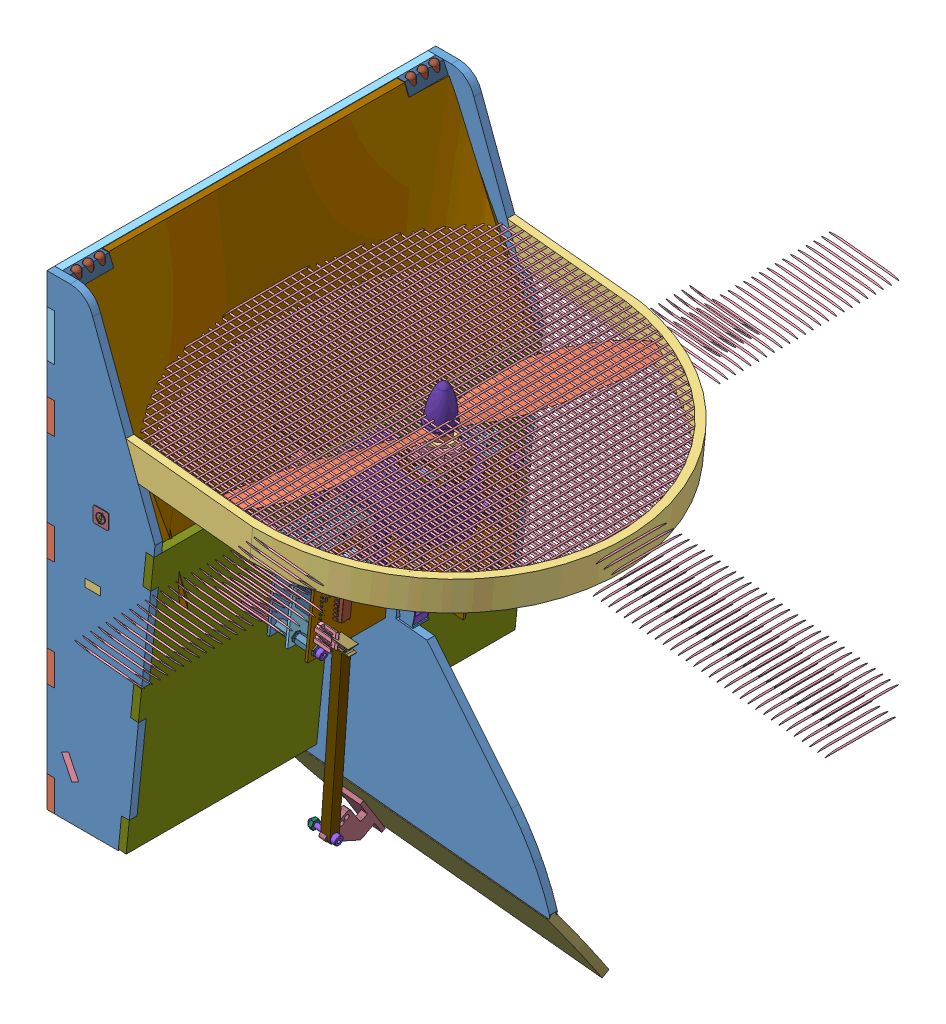
SolidWorks assembly AssTotaleSimu5, configuration Défaut. Lengths in mm. (continued)
Components (placement in the parent): (continued)
- AssStructSimu-1: AssStructSimu [Défaut] at (-125.7658 -1.8483 624.6548) x (1 0 0) z (0 0 -1) size (253.25 324.59 251.6) (continued)
  - AssCarte-1: AssCarte [Défaut] at (38.0121 147.1029 290.772) x (-0.101852 0.9948 0) z (0.9948 0.101852 0) size (66.52 130.57 98.72) (continued)
    - carte_onduleur_v3-1: carte_onduleur_v3 [Défaut] at (-131.8199 12.0892 20.7912) size (66.52 130.57 82.34) (continued)
      - RC2_2-1: RC2_2 [Défaut] at (-22 0.18 -0.803) x (-1 0 0) z (0 0 -1) size (2.34 1.04 0.5) (continued)
        - Open CASCADE STEP translator 6.8 1.12.1-1: Open CASCADE STEP translator 6.8 1.12.1 [Défaut] at origin size (2.34 1.04 0.5) (continued)
          - Pin_2_2-1: Pin_2_2 [Défaut] at origin size (0.51 1.02 0.5)
      - RC3_1-1: RC3_1 [Défaut] at (-20.9336 -14.5 -0.803) x (1 0 0) z (0 0 -1) size (2.34 1.04 0.5)
        - Open CASCADE STEP translator 6.8 1.12.1-1: Open CASCADE STEP translator 6.8 1.12.1 [Défaut] at origin size (2.34 1.04 0.5)
          - Body_1_3-1: Body_1_3 [Défaut] at origin size (2.29 1.04 0.43)
          - Pin_1_2-1: Pin_1_2 [Défaut] at (0.3048 0 0) x (-1 0 0) z (0 0 1) size (0.51 1.02 0.5)
          - Pin_2_2-1: Pin_2_2 [Défaut] at origin size (0.51 1.02 0.5)
      - RC3_2-1: RC3_2 [Défaut] at (-22.3 -14.5 -0.803) x (-1 0 0) z (0 0 -1) size (2.34 1.04 0.5)
        - Open CASCADE STEP translator 6.8 1.12.1-1: Open CASCADE STEP translator 6.8 1.12.1 [Défaut] at origin size (2.34 1.04 0.5)
          - Body_1_3-1: Body_1_3 [Défaut] at origin size (2.29 1.04 0.43)
          - Pin_1_2-1: Pin_1_2 [Défaut] at (0.3048 0 0) x (-1 0 0) z (0 0 1) size (0.51 1.02 0.5)
          - Pin_2_2-1: Pin_2_2 [Défaut] at origin size (0.51 1.02 0.5)
      - U_MES_CUR-1: U_MES_CUR [Défaut] at (-11.5 6.7816 0.803) size (2.54 2.41 0.76)
        - Open CASCADE STEP translator 6.8 1.32.1-1: Open CASCADE STEP translator 6.8 1.32.1 [Défaut] at origin size (2.54 2.41 0.76)
          - Body_1_5-1: Body_1_5 [Défaut] at origin size (2.54 1.27 0.71)
          - Pin_1_3-1: Pin_1_3 [Défaut] at (-2.1082 0.2286 0) x (0 -1 0) z (0 0 1) size (1.14 0.25 0.47)
          - Pin_2_3-1: Pin_2_3 [Défaut] at (-0.2032 2.1336 0) x (0 -1 0) z (0 0 1) size (1.14 0.25 0.47)
      - CARTE_ALIM-1: CARTE_ALIM [Défaut] at (-6.4 -57.2 0.803) size (60 130 18.35)
        - Open CASCADE STEP translator 6.8 1.33.1-1: Open CASCADE STEP translator 6.8 1.33.1 [Défaut] at origin size (60 130 18.35)
          - Body_1_6-1: Body_1_6 [Défaut] at (7 56 -12) size (60 130 18.35)
            - 1_3-1: 1_3 [Défaut] at origin size (60 130 1.61)
            - 13_3-1: 13_3 [Défaut] at (0.4717 -40.93 0.803) x (0 1 0) z (0 0 1) size (5.65 4.9 1.7)
              - =_[0_1_1_4]_3-1: =_[0_1_1_4]_3 [Défaut] at origin size (5.65 4.9 1.7)
                - 2-1: 2 [Défaut] at origin size (3.75 4.9 1.53)
                - 3-1: 3 [Défaut] at origin size (0.95 0.51 1.06)
                - 4-1: 4 [Défaut] at origin size (0.95 0.51 1.06)
                - 5_2-1: 5_2 [Défaut] at origin size (0.95 0.51 1.06)
                - 6-1: 6 [Défaut] at origin size (0.95 0.51 1.06)
                - 7-1: 7 [Défaut] at (10.8 -5.08 0) x (-1 0 0) z (0 0 1) size (0.95 0.51 1.06)
                - 8_2-1: 8_2 [Défaut] at (10.8 -2.54 0) x (-1 0 0) z (0 0 1) size (0.95 0.51 1.06)
                - 9-1: 9 [Défaut] at (10.8 0 0) x (-1 0 0) z (0 0 1) size (0.95 0.51 1.06)
                - 10-1: 10 [Défaut] at (10.8 2.54 0) x (-1 0 0) z (0 0 1) size (0.95 0.51 1.06)
                - 11_2-1: 11_2 [Défaut] at (5.4 -1.27 0) x (-1 0 0) z (0 0 1) size (4.25 2.34 1.06)
            - 18-1: 18 [Défaut] at (-2.5283 -37.23 0.803) x (0 -1 0) z (0 0 1) size (2.34 1.04 0.5)
              - =_[0_1_1_16]-1: =_[0_1_1_16] [Défaut] at origin size (2.34 1.04 0.5)
                - 14_2-1: 14_2 [Défaut] at origin size (2.29 1.04 0.43)
                - 15_2-1: 15_2 [Défaut] at (0.3048 0 0) x (-1 0 0) z (0 0 1) size (0.51 1.02 0.5)
                - 16_2-1: 16_2 [Défaut] at origin size (0.51 1.02 0.5)
            - 21_2-1: 21_2 [Défaut] at (-2.2263 -24.628 -0.803) x (1 0 0) z (0 0 -1) size (8.01 8 14.24)
              - =_[0_1_1_21]-1: =_[0_1_1_21] [Défaut] at origin size (8.01 8 14.24)
                - 19-1: 19 [Défaut] at (1.8 0 0) x (1 0 0) z (0 -1 0) size (8.01 14.24 8)
            - 23_2-1: 23_2 [Défaut] at (1.2381 -31.53 0.803) size (2.34 1.04 0.5)
              - =_[0_1_1_16]-1: =_[0_1_1_16] [Défaut] at origin size (2.34 1.04 0.5)
                - 14_2-1: 14_2 [Défaut] at origin size (2.29 1.04 0.43)
                - 15_2-1: 15_2 [Défaut] at (0.3048 0 0) x (-1 0 0) z (0 0 1) size (0.51 1.02 0.5)
                - 16_2-1: 16_2 [Défaut] at origin size (0.51 1.02 0.5)
            - 28-1: 28 [Défaut] at (5 29.8636 0.803) x (0 -1 0) z (0 0 1) size (3.35 1.3 0.55)
              - =_[0_1_1_25]_2-1: =_[0_1_1_25]_2 [Défaut] at origin size (3.35 1.3 0.55)
                - 24-1: 24 [Défaut] at origin size (3.3 1.3 0.48)
                - 25_2-1: 25_2 [Défaut] at (0.5588 0 0) x (-1 0 0) z (0 0 1) size (0.76 1.27 0.55)
                - 26_2-1: 26_2 [Défaut] at origin size (0.76 1.27 0.55)
            - 30-1: 30 [Défaut] at (6.7 29.8636 0.803) x (0 -1 0) z (0 0 1) size (2.34 1.04 0.5)
              - =_[0_1_1_16]-1: =_[0_1_1_16] [Défaut] at origin size (2.34 1.04 0.5)
                - 14_2-1: 14_2 [Défaut] at origin size (2.29 1.04 0.43)
                - 15_2-1: 15_2 [Défaut] at (0.3048 0 0) x (-1 0 0) z (0 0 1) size (0.51 1.02 0.5)
                - 16_2-1: 16_2 [Défaut] at origin size (0.51 1.02 0.5)
            - 35_2-1: 35_2 [Défaut] at (-2.5 -46.37 0.803) x (0 1 0) z (0 0 1) size (3.4 2.06 0.79)
              - =_[0_1_1_31]-1: =_[0_1_1_31] [Défaut] at origin size (3.4 2.06 0.79)
                - 31_2-1: 31_2 [Défaut] at origin size (3.3 2.06 0.69)
                - 32_3-1: 32_3 [Défaut] at (0.5588 0 0) x (-1 0 0) z (0 0 1) size (0.81 2.03 0.79)
                - 33_3-1: 33_3 [Défaut] at origin size (0.81 2.03 0.79)
            - 37-1: 37 [Défaut] at (5 31.43 0.803) x (0 1 0) z (0 0 1) size (2.34 1.04 0.5)
              - =_[0_1_1_16]-1: =_[0_1_1_16] [Défaut] at origin size (2.34 1.04 0.5)
                - 14_2-1: 14_2 [Défaut] at origin size (2.29 1.04 0.43)
                - 15_2-1: 15_2 [Défaut] at (0.3048 0 0) x (-1 0 0) z (0 0 1) size (0.51 1.02 0.5)
                - 16_2-1: 16_2 [Défaut] at origin size (0.51 1.02 0.5)
            - 39-1: 39 [Défaut] at (-0.2 35.63 0.803) x (-1 0 0) z (0 0 1) size (2.34 1.04 0.5)
              - =_[0_1_1_16]-1: =_[0_1_1_16] [Défaut] at origin size (2.34 1.04 0.5)
                - 14_2-1: 14_2 [Défaut] at origin size (2.29 1.04 0.43)
                - 15_2-1: 15_2 [Défaut] at (0.3048 0 0) x (-1 0 0) z (0 0 1) size (0.51 1.02 0.5)
                - 16_2-1: 16_2 [Défaut] at origin size (0.51 1.02 0.5)
            - 41-1: 41 [Défaut] at (2.9 -45.5036 0.803) x (0 1 0) z (0 0 1) size (2.34 1.04 0.5)
              - =_[0_1_1_16]-1: =_[0_1_1_16] [Défaut] at origin size (2.34 1.04 0.5)
                - 14_2-1: 14_2 [Défaut] at origin size (2.29 1.04 0.43)
                - 15_2-1: 15_2 [Défaut] at (0.3048 0 0) x (-1 0 0) z (0 0 1) size (0.51 1.02 0.5)
                - 16_2-1: 16_2 [Défaut] at origin size (0.51 1.02 0.5)
            - 43-1: 43 [Défaut] at (17.1348 -42.6272 0.803) x (0 1 0) z (0 0 1) size (2.34 1.04 0.5)
              - =_[0_1_1_16]-1: =_[0_1_1_16] [Défaut] at origin size (2.34 1.04 0.5)
                - 14_2-1: 14_2 [Défaut] at origin size (2.29 1.04 0.43)
                - 15_2-1: 15_2 [Défaut] at (0.3048 0 0) x (-1 0 0) z (0 0 1) size (0.51 1.02 0.5)
                - 16_2-1: 16_2 [Défaut] at origin size (0.51 1.02 0.5)
            - 48_2-1: 48_2 [Défaut] at (-5.4717 -39.01 0.803) x (-1 0 0) z (0 0 1) size (4.19 3.4 1.75)
              - =_[0_1_1_40]-1: =_[0_1_1_40] [Défaut] at origin size (4.19 3.4 1.75)
                - 44_2-1: 44_2 [Défaut] at origin size (3.75 3.38 1.73)
                - 45_2-1: 45_2 [Défaut] at (0.438 0 0) x (-1 0 0) z (0 0 1) size (0.53 3.4 1.75)
                - 46_2-1: 46_2 [Défaut] at origin size (0.52 3.4 1.75)
            - 53-1: 53 [Défaut] at (0.9 35.63 0.803) size (2.34 1.04 0.5)
              - =_[0_1_1_45]-1: =_[0_1_1_45] [Défaut] at origin size (2.34 1.04 0.5)
                - 49_3-1: 49_3 [Défaut] at origin size (2.29 1.04 0.43)
                - 50-1: 50 [Défaut] at (0.3048 0 0) x (-1 0 0) z (0 0 1) size (0.51 1.02 0.5)
                - 51-1: 51 [Défaut] at origin size (0.51 1.02 0.5)
            - 55_2-1: 55_2 [Défaut] at (1.3 -45.5036 0.803) x (0 1 0) z (0 0 1) size (2.34 1.04 0.5)
              - =_[0_1_1_45]-1: =_[0_1_1_45] [Défaut] at origin size (2.34 1.04 0.5)
                - 49_3-1: 49_3 [Défaut] at origin size (2.29 1.04 0.43)
                - 50-1: 50 [Défaut] at (0.3048 0 0) x (-1 0 0) z (0 0 1) size (0.51 1.02 0.5)
                - 51-1: 51 [Défaut] at origin size (0.51 1.02 0.5)
            - 57_3-1: 57_3 [Défaut] at (17.2348 -43.9936 0.803) x (0 -1 0) z (0 0 1) size (2.34 1.04 0.5)
              - =_[0_1_1_45]-1: =_[0_1_1_45] [Défaut] at origin size (2.34 1.04 0.5)
                - 49_3-1: 49_3 [Défaut] at origin size (2.29 1.04 0.43)
                - 50-1: 50 [Défaut] at (0.3048 0 0) x (-1 0 0) z (0 0 1) size (0.51 1.02 0.5)
                - 51-1: 51 [Défaut] at origin size (0.51 1.02 0.5)
            - 65-1: 65 [Défaut] at (-4.8 30.93 0.803) x (-1 0 0) z (0 0 1) size (14.64 9.83 4.25)
              - =_[0_1_1_52]-1: =_[0_1_1_52] [Défaut] at origin size (14.64 9.83 4.25)
                - 63_2-1: 63_2 [Défaut] at (3 0 0) x (0 -1 0) z (0 0 1) size (9.83 14.64 4.25)
                  - =_[0_1_1_3]_5-1: =_[0_1_1_3]_5 [Défaut] at origin size (9.83 9.05 4.21)
                  - =_[0_1_1_4]_5-1: =_[0_1_1_4]_5 [Défaut] at origin size (9.48 7.76 1.21)
                  - =_[0_1_1_5]_5-1: =_[0_1_1_5]_5 [Défaut] at origin size (1.36 6.01 3.08)
                  - =_[0_1_1_6]_3-1: =_[0_1_1_6]_3 [Défaut] at origin size (1.36 6.01 3.08)
                  - =_[0_1_1_7]_3-1: =_[0_1_1_7]_3 [Défaut] at origin size (1.06 6.01 3.08)
            - 67-1: 67 [Défaut] at (13.5933 -37.5272 0.803) x (-1 0 0) z (0 0 1) size (2.34 1.04 0.5)
              - =_[0_1_1_16]-1: =_[0_1_1_16] [Défaut] at origin size (2.34 1.04 0.5)
                - 14_2-1: 14_2 [Défaut] at origin size (2.29 1.04 0.43)
                - 15_2-1: 15_2 [Défaut] at (0.3048 0 0) x (-1 0 0) z (0 0 1) size (0.51 1.02 0.5)
                - 16_2-1: 16_2 [Défaut] at origin size (0.51 1.02 0.5)
            - 70_2-1: 70_2 [Défaut] at (18.2733 -29.7272 0.803) x (0 1 0) z (0 0 1) size (6.06 4.95 1.88)
              - =_[0_1_1_61]-1: =_[0_1_1_61] [Défaut] at origin size (6.06 4.95 1.88)
                - 68-1: 68 [Défaut] x (1 0 0) z (0 -1 0) size (6.06 1.88 4.95)
            - 83-1: 83 [Défaut] at (-21.2 -38.07 0.803) x (-1 0 0) z (0 0 1) size (2.7 5.2 1.11)
              - =_[0_1_1_64]-1: =_[0_1_1_64] [Défaut] at origin size (2.7 5.2 1.11)
                - 84_2-1: 84_2 [Défaut] at (1.2 -4 0) x (0 1 0) z (0 0 1) size (5.2 2.7 1.11)
                  - =_[0_1_1_3]_6-1: =_[0_1_1_3]_6 [Défaut] at origin size (0.39 0.64 0.01)
                  - =_[0_1_1_4]_6-1: =_[0_1_1_4]_6 [Défaut] at origin size (0.6 1.9 0.2)
                  - =_[0_1_1_5]_6-1: =_[0_1_1_5]_6 [Défaut] at origin size (0.21 0.08 0.01)
                  - =_[0_1_1_6]_4-1: =_[0_1_1_6]_4 [Défaut] at origin size (0.6 1.9 0.2)
                  - =_[0_1_1_7]_4-1: =_[0_1_1_7]_4 [Défaut] at origin size (0.46 0.68 0.01)
                  - =_[0_1_1_8]_3-1: =_[0_1_1_8]_3 [Défaut] at origin size (0.38 0.66 0.01)
                  - =_[0_1_1_9]_2-1: =_[0_1_1_9]_2 [Défaut] at origin size (0.2 0.62 0.01)
                  - =_[0_1_1_10]_2-1: =_[0_1_1_10]_2 [Défaut] at origin size (4 2.7 1.1)
                  - =_[0_1_1_11]_2-1: =_[0_1_1_11]_2 [Défaut] at origin size (0.46 0.63 0.01)
                  - =_[0_1_1_12]_2-1: =_[0_1_1_12]_2 [Défaut] at origin size (0.56 0.68 0.01)
            - 86_2-1: 86_2 [Défaut] at (12.8933 -35.4272 0.803) x (0 1 0) z (0 0 1) size (2.7 5.2 1.11)
              - =_[0_1_1_77]-1: =_[0_1_1_77] [Défaut] at origin size (2.7 5.2 1.11)
                - 84_2-1: 84_2 [Défaut] at (1.2 -4 0) x (0 1 0) z (0 0 1) size (5.2 2.7 1.11)
                  - =_[0_1_1_3]_6-1: =_[0_1_1_3]_6 [Défaut] at origin size (0.39 0.64 0.01)
                  - =_[0_1_1_4]_6-1: =_[0_1_1_4]_6 [Défaut] at origin size (0.6 1.9 0.2)
                  - =_[0_1_1_5]_6-1: =_[0_1_1_5]_6 [Défaut] at origin size (0.21 0.08 0.01)
                  - =_[0_1_1_6]_4-1: =_[0_1_1_6]_4 [Défaut] at origin size (0.6 1.9 0.2)
                  - =_[0_1_1_7]_4-1: =_[0_1_1_7]_4 [Défaut] at origin size (0.46 0.68 0.01)
                  - =_[0_1_1_8]_3-1: =_[0_1_1_8]_3 [Défaut] at origin size (0.38 0.66 0.01)
                  - =_[0_1_1_9]_2-1: =_[0_1_1_9]_2 [Défaut] at origin size (0.2 0.62 0.01)
                  - =_[0_1_1_10]_2-1: =_[0_1_1_10]_2 [Défaut] at origin size (4 2.7 1.1)
                  - =_[0_1_1_11]_2-1: =_[0_1_1_11]_2 [Défaut] at origin size (0.46 0.63 0.01)
                  - =_[0_1_1_12]_2-1: =_[0_1_1_12]_2 [Défaut] at origin size (0.56 0.68 0.01)
            - 92_2-1: 92_2 [Défaut] at (20.9933 -39.3272 0.803) x (0 -1 0) z (0 0 1) size (2.79 1.98 0.64)
              - =_[0_1_1_79]-1: =_[0_1_1_79] [Défaut] at origin size (2.79 1.98 0.64)
                - 87-1: 87 [Défaut] at origin size (2.79 1.02 0.58)
                - 88-1: 88 [Défaut] x (0 -1 0) z (0 0 1) size (0.42 0.38 0.38)
                - 89-1: 89 [Défaut] at (-2.8448 -0.9652 0) x (0 1 0) z (0 0 1) size (0.55 0.38 0.38)
                - 90-1: 90 [Défaut] at (-0.9652 -2.8448 0) x (0 1 0) z (0 0 1) size (0.55 0.38 0.38)
            - 98-1: 98 [Défaut] at (-17.7 -48.47 0.803) x (0 -1 0) z (0 0 1) size (2.54 1.98 0.64)
              - =_[0_1_1_85]-1: =_[0_1_1_85] [Défaut] at origin size (2.54 1.98 0.64)
                - 93-1: 93 [Défaut] at origin size (2.54 1.14 0.58)
                - 94-1: 94 [Défaut] x (0 -1 0) z (0 0 1) size (0.43 0.51 0.38)
                - 95-1: 95 [Défaut] at (1.8796 1.8796 0) x (0 -1 0) z (0 0 1) size (0.43 0.51 0.38)
                - 96-1: 96 [Défaut] at (-0.9652 -2.8448 0) x (0 1 0) z (0 0 1) size (0.41 0.51 0.38)
            - 100-1: 100 [Défaut] at (24.3933 -43.2272 0.803) size (2.79 1.98 0.64)
              - =_[0_1_1_79]-1: =_[0_1_1_79] [Défaut] at origin size (2.79 1.98 0.64)
                - 87-1: 87 [Défaut] at origin size (2.79 1.02 0.58)
                - 88-1: 88 [Défaut] x (0 -1 0) z (0 0 1) size (0.42 0.38 0.38)
                - 89-1: 89 [Défaut] at (-2.8448 -0.9652 0) x (0 1 0) z (0 0 1) size (0.55 0.38 0.38)
                - 90-1: 90 [Défaut] at (-0.9652 -2.8448 0) x (0 1 0) z (0 0 1) size (0.55 0.38 0.38)
            - 102-1: 102 [Défaut] at (21.4933 -44.4272 0.803) x (0 -1 0) z (0 0 1) size (2.79 1.98 0.64)
              - =_[0_1_1_79]-1: =_[0_1_1_79] [Défaut] at origin size (2.79 1.98 0.64)
                - 87-1: 87 [Défaut] at origin size (2.79 1.02 0.58)
                - 88-1: 88 [Défaut] x (0 -1 0) z (0 0 1) size (0.42 0.38 0.38)
                - 89-1: 89 [Défaut] at (-2.8448 -0.9652 0) x (0 1 0) z (0 0 1) size (0.55 0.38 0.38)
                - 90-1: 90 [Défaut] at (-0.9652 -2.8448 0) x (0 1 0) z (0 0 1) size (0.55 0.38 0.38)
            - 107-1: 107 [Défaut] at (23.1933 -29.1272 -0.803) x (0 1 0) z (0 0 -1) size (9.6 14.35 5)
              - =_[0_1_1_93]-1: =_[0_1_1_93] [Défaut] at origin size (9.6 14.35 5)
                - 105-1: 105 [Défaut] at (0.5 -1 2) x (-1 0 0) z (0 0 1) size (9.6 14.35 5)
                  - =_[0_1_1_3]_7-1: =_[0_1_1_3]_7 [Défaut] at origin size (9.6 12.75 5)
                  - =_[0_1_1_4]_7-1: =_[0_1_1_4]_7 [Défaut] at origin size (2.2 1.6 2.2)
            - 109-1: 109 [Défaut] at (25.4933 -41.1272 0.803) x (-1 0 0) z (0 0 1) size (2.34 1.04 0.5)
              - =_[0_1_1_45]-1: =_[0_1_1_45] [Défaut] at origin size (2.34 1.04 0.5)
                - 49_3-1: 49_3 [Défaut] at origin size (2.29 1.04 0.43)
                - 50-1: 50 [Défaut] at (0.3048 0 0) x (-1 0 0) z (0 0 1) size (0.51 1.02 0.5)
                - 51-1: 51 [Défaut] at origin size (0.51 1.02 0.5)
            - 111-1: 111 [Défaut] at (22.0269 -41.8272 0.803) x (-1 0 0) z (0 0 1) size (2.34 1.04 0.5)
              - =_[0_1_1_45]-1: =_[0_1_1_45] [Défaut] at origin size (2.34 1.04 0.5)
                - 49_3-1: 49_3 [Défaut] at origin size (2.29 1.04 0.43)
                - 50-1: 50 [Défaut] at (0.3048 0 0) x (-1 0 0) z (0 0 1) size (0.51 1.02 0.5)
                - 51-1: 51 [Défaut] at origin size (0.51 1.02 0.5)
            - 113-1: 113 [Défaut] at (-24.8 -36.7036 0.803) x (0 1 0) z (0 0 1) size (2.34 1.04 0.5)
              - =_[0_1_1_45]-1: =_[0_1_1_45] [Défaut] at origin size (2.34 1.04 0.5)
                - 49_3-1: 49_3 [Défaut] at origin size (2.29 1.04 0.43)
                - 50-1: 50 [Défaut] at (0.3048 0 0) x (-1 0 0) z (0 0 1) size (0.51 1.02 0.5)
                - 51-1: 51 [Défaut] at origin size (0.51 1.02 0.5)
            - 115-1: 115 [Défaut] at (-24.8 -40.3036 0.803) x (0 1 0) z (0 0 1) size (2.34 1.04 0.5)
              - =_[0_1_1_45]-1: =_[0_1_1_45] [Défaut] at origin size (2.34 1.04 0.5)
                - 49_3-1: 49_3 [Défaut] at origin size (2.29 1.04 0.43)
                - 50-1: 50 [Défaut] at (0.3048 0 0) x (-1 0 0) z (0 0 1) size (0.51 1.02 0.5)
                - 51-1: 51 [Défaut] at origin size (0.51 1.02 0.5)
            - 117-1: 117 [Défaut] at (-16 -48.27 0.803) x (0 -1 0) z (0 0 1) size (2.34 1.04 0.5)
              - =_[0_1_1_45]-1: =_[0_1_1_45] [Défaut] at origin size (2.34 1.04 0.5)
                - 49_3-1: 49_3 [Défaut] at origin size (2.29 1.04 0.43)
                - 50-1: 50 [Défaut] at (0.3048 0 0) x (-1 0 0) z (0 0 1) size (0.51 1.02 0.5)
                - 51-1: 51 [Défaut] at origin size (0.51 1.02 0.5)
            - 119-1: 119 [Défaut] at (-22.5189 -47.87 0.803) x (-1 0 0) z (0 0 1) size (2.34 1.04 0.5)
              - =_[0_1_1_45]-1: =_[0_1_1_45] [Défaut] at origin size (2.34 1.04 0.5)
                - 49_3-1: 49_3 [Défaut] at origin size (2.29 1.04 0.43)
                - 50-1: 50 [Défaut] at (0.3048 0 0) x (-1 0 0) z (0 0 1) size (0.51 1.02 0.5)
                - 51-1: 51 [Défaut] at origin size (0.51 1.02 0.5)
            - 121-1: 121 [Défaut] at (22.3933 -38.9272 0.803) size (2.34 1.04 0.5)
              - =_[0_1_1_45]-1: =_[0_1_1_45] [Défaut] at origin size (2.34 1.04 0.5)
                - 49_3-1: 49_3 [Défaut] at origin size (2.29 1.04 0.43)
                - 50-1: 50 [Défaut] at (0.3048 0 0) x (-1 0 0) z (0 0 1) size (0.51 1.02 0.5)
                - 51-1: 51 [Défaut] at origin size (0.51 1.02 0.5)
            - 123-1: 123 [Défaut] at (22.0933 -36.4272 0.803) x (-1 0 0) z (0 0 1) size (2.34 1.04 0.5)
              - =_[0_1_1_45]-1: =_[0_1_1_45] [Défaut] at origin size (2.34 1.04 0.5)
                - 49_3-1: 49_3 [Défaut] at origin size (2.29 1.04 0.43)
                - 50-1: 50 [Défaut] at (0.3048 0 0) x (-1 0 0) z (0 0 1) size (0.51 1.02 0.5)
                - 51-1: 51 [Défaut] at origin size (0.51 1.02 0.5)
            - 125-1: 125 [Défaut] at (22.3933 -32.0272 0.803) x (0 -1 0) z (0 0 1) size (2.34 1.04 0.5)
              - =_[0_1_1_45]-1: =_[0_1_1_45] [Défaut] at origin size (2.34 1.04 0.5)
                - 49_3-1: 49_3 [Défaut] at origin size (2.29 1.04 0.43)
                - 50-1: 50 [Défaut] at (0.3048 0 0) x (-1 0 0) z (0 0 1) size (0.51 1.02 0.5)
                - 51-1: 51 [Défaut] at origin size (0.51 1.02 0.5)
            - 127-1: 127 [Défaut] at (17.9597 -23.1272 0.803) size (2.34 1.04 0.5)
              - =_[0_1_1_16]-1: =_[0_1_1_16] [Défaut] at origin size (2.34 1.04 0.5)
                - 14_2-1: 14_2 [Défaut] at origin size (2.29 1.04 0.43)
                - 15_2-1: 15_2 [Défaut] at (0.3048 0 0) x (-1 0 0) z (0 0 1) size (0.51 1.02 0.5)
                - 16_2-1: 16_2 [Défaut] at origin size (0.51 1.02 0.5)
            - 129-1: 129 [Défaut] at (20.0269 -24.9272 0.803) x (-1 0 0) z (0 0 1) size (2.34 1.04 0.5)
              - =_[0_1_1_16]-1: =_[0_1_1_16] [Défaut] at origin size (2.34 1.04 0.5)
                - 14_2-1: 14_2 [Défaut] at origin size (2.29 1.04 0.43)
                - 15_2-1: 15_2 [Défaut] at (0.3048 0 0) x (-1 0 0) z (0 0 1) size (0.51 1.02 0.5)
                - 16_2-1: 16_2 [Défaut] at origin size (0.51 1.02 0.5)
            - 131-1: 131 [Défaut] at (16.9933 -37.5272 0.803) x (-1 0 0) z (0 0 1) size (2.34 1.04 0.5)
              - =_[0_1_1_45]-1: =_[0_1_1_45] [Défaut] at origin size (2.34 1.04 0.5)
                - 49_3-1: 49_3 [Défaut] at origin size (2.29 1.04 0.43)
                - 50-1: 50 [Défaut] at (0.3048 0 0) x (-1 0 0) z (0 0 1) size (0.51 1.02 0.5)
                - 51-1: 51 [Défaut] at origin size (0.51 1.02 0.5)
            - 136-1: 136 [Défaut] at (3.2957 -29.23 0.803) x (-1 0 0) z (0 0 1) size (4.78 2.79 2.03)
              - =_[0_1_1_110]_2-1: =_[0_1_1_110]_2 [Défaut] at origin size (4.78 2.79 2.03)
                - 132-1: 132 [Défaut] at origin size (4.32 2.79 1.78)
                - 133-1: 133 [Défaut] at (0.4572 0 0) x (-1 0 0) z (0 0 1) size (1.02 1.27 1.32)
                - 134-1: 134 [Défaut] at origin size (1.02 1.27 1.32)
            - 141-1: 141 [Défaut] at (0.2436 -33.3673 0.803) size (3.35 1.3 0.55)
              - =_[0_1_1_115]_2-1: =_[0_1_1_115]_2 [Défaut] at origin size (3.35 1.3 0.55)
                - 137-1: 137 [Défaut] at origin size (3.3 1.3 0.48)
                - 138-1: 138 [Défaut] at (0.5588 0 0) x (-1 0 0) z (0 0 1) size (0.76 1.27 0.55)
                - 139-1: 139 [Défaut] at origin size (0.76 1.27 0.55)
            - 143_2-1: 143_2 [Défaut] at (-0.3 -45.47 0.803) x (0 1 0) z (0 0 1) size (2.34 1.04 0.5)
              - =_[0_1_1_16]-1: =_[0_1_1_16] [Défaut] at origin size (2.34 1.04 0.5)
                - 14_2-1: 14_2 [Défaut] at origin size (2.29 1.04 0.43)
                - 15_2-1: 15_2 [Défaut] at (0.3048 0 0) x (-1 0 0) z (0 0 1) size (0.51 1.02 0.5)
                - 16_2-1: 16_2 [Défaut] at origin size (0.51 1.02 0.5)
            - 145-1: 145 [Défaut] at (6.6 31.13 0.803) x (0 1 0) z (0 0 1) size (3.35 1.3 0.55)
              - =_[0_1_1_25]_2-1: =_[0_1_1_25]_2 [Défaut] at origin size (3.35 1.3 0.55)
                - 24-1: 24 [Défaut] at origin size (3.3 1.3 0.48)
                - 25_2-1: 25_2 [Défaut] at (0.5588 0 0) x (-1 0 0) z (0 0 1) size (0.76 1.27 0.55)
                - 26_2-1: 26_2 [Défaut] at origin size (0.76 1.27 0.55)
            - 148-1: 148 [Défaut] at (-7.5 -56.57 0.803) size (15.24 2.54 7.37)
              - =_[0_1_1_122]_2-1: =_[0_1_1_122]_2 [Défaut] at origin size (15.24 2.54 7.37)
                - 146-1: 146 [Défaut] at (6.3 0 1) x (1 0 0) z (0 -1 0) size (15.24 7.37 2.54)
      - COMP1-1: COMP1 [Défaut] at (-16.3 -36.2 0.803) x (-1 0 0) z (0 0 1) size (2.03 1.88 0.51)
        - Open CASCADE STEP translator 6.8 1.34.1-1: Open CASCADE STEP translator 6.8 1.34.1 [Défaut] at origin size (2.03 1.88 0.51)
          - Body_1_6-1: Body_1_6 [Défaut] at origin size (2.03 1.02 0.46)
          - Pin_1_4-1: Pin_1_4 [Défaut] x (0 1 0) z (0 0 1) size (0.45 0.25 0.32)
          - Pin_2_4-1: Pin_2_4 [Défaut] at (0.65 -0.65 0) x (0 1 0) z (0 0 1) size (0.45 0.25 0.32)
          - Pin_3-1: Pin_3 [Défaut] at (1.3 -1.3 0) x (0 1 0) z (0 0 1) size (0.45 0.25 0.32)
          - Pin_4-1: Pin_4 [Défaut] at (-0.5 3.1 0) x (0 -1 0) z (0 0 1) size (0.41 0.25 0.32)
          - Pin_5-1: Pin_5 [Défaut] at (-1.8 1.8 0) x (0 -1 0) z (0 0 1) size (0.41 0.25 0.32)
      - COMP2-1: COMP2 [Défaut] at (-14.3 -9.6 0.803) x (-1 0 0) z (0 0 1) size (2.03 1.88 0.51)
        - Open CASCADE STEP translator 6.8 1.34.1-1: Open CASCADE STEP translator 6.8 1.34.1 [Défaut] at origin size (2.03 1.88 0.51)
          - Body_1_6-1: Body_1_6 [Défaut] at origin size (2.03 1.02 0.46)
          - Pin_1_4-1: Pin_1_4 [Défaut] x (0 1 0) z (0 0 1) size (0.45 0.25 0.32)
          - Pin_2_4-1: Pin_2_4 [Défaut] at (0.65 -0.65 0) x (0 1 0) z (0 0 1) size (0.45 0.25 0.32)
          - Pin_3-1: Pin_3 [Défaut] at (1.3 -1.3 0) x (0 1 0) z (0 0 1) size (0.45 0.25 0.32)
          - Pin_4-1: Pin_4 [Défaut] at (-0.5 3.1 0) x (0 -1 0) z (0 0 1) size (0.41 0.25 0.32)
          - Pin_5-1: Pin_5 [Défaut] at (-1.8 1.8 0) x (0 -1 0) z (0 0 1) size (0.41 0.25 0.32)
      - COMP3-1: COMP3 [Défaut] at (-15.9 -23.2 0.803) x (-1 0 0) z (0 0 1) size (2.03 1.88 0.51)
        - Open CASCADE STEP translator 6.8 1.34.1-1: Open CASCADE STEP translator 6.8 1.34.1 [Défaut] at origin size (2.03 1.88 0.51)
          - Body_1_6-1: Body_1_6 [Défaut] at origin size (2.03 1.02 0.46)
          - Pin_1_4-1: Pin_1_4 [Défaut] x (0 1 0) z (0 0 1) size (0.45 0.25 0.32)
          - Pin_2_4-1: Pin_2_4 [Défaut] at (0.65 -0.65 0) x (0 1 0) z (0 0 1) size (0.45 0.25 0.32)
          - Pin_3-1: Pin_3 [Défaut] at (1.3 -1.3 0) x (0 1 0) z (0 0 1) size (0.45 0.25 0.32)
          - Pin_4-1: Pin_4 [Défaut] at (-0.5 3.1 0) x (0 -1 0) z (0 0 1) size (0.41 0.25 0.32)
          - Pin_5-1: Pin_5 [Défaut] at (-1.8 1.8 0) x (0 -1 0) z (0 0 1) size (0.41 0.25 0.32)
      - CP1-1: CP1 [Défaut] at (-18.9 -38.2 0.803) x (0 1 0) z (0 0 1) size (2.34 1.04 0.5)
        - Open CASCADE STEP translator 6.8 1.6.1-1: Open CASCADE STEP translator 6.8 1.6.1 [Défaut] at origin size (2.34 1.04 0.5)
          - Body_1-1: Body_1 [Défaut] at origin size (2.29 1.04 0.43)
          - Pin_1-1: Pin_1 [Défaut] at (0.3048 0 0) x (-1 0 0) z (0 0 1) size (0.51 1.02 0.5)
          - Pin_2-1: Pin_2 [Défaut] at origin size (0.51 1.02 0.5)
      - CP2-1: CP2 [Défaut] at (-16.9 -11.6 0.803) x (0 1 0) z (0 0 1) size (2.34 1.04 0.5)
        - Open CASCADE STEP translator 6.8 1.6.1-1: Open CASCADE STEP translator 6.8 1.6.1 [Défaut] at origin size (2.34 1.04 0.5)
          - Body_1-1: Body_1 [Défaut] at origin size (2.29 1.04 0.43)
          - Pin_1-1: Pin_1 [Défaut] at (0.3048 0 0) x (-1 0 0) z (0 0 1) size (0.51 1.02 0.5)
          - Pin_2-1: Pin_2 [Défaut] at origin size (0.51 1.02 0.5)
      - CP3-1: CP3 [Défaut] at (-18.5 -25.2 0.803) x (0 1 0) z (0 0 1) size (2.34 1.04 0.5)
        - Open CASCADE STEP translator 6.8 1.6.1-1: Open CASCADE STEP translator 6.8 1.6.1 [Défaut] at origin size (2.34 1.04 0.5)
          - Body_1-1: Body_1 [Défaut] at origin size (2.29 1.04 0.43)
          - Pin_1-1: Pin_1 [Défaut] at (0.3048 0 0) x (-1 0 0) z (0 0 1) size (0.51 1.02 0.5)
          - Pin_2-1: Pin_2 [Défaut] at origin size (0.51 1.02 0.5)
      - C_DEC_COM1-1: C_DEC_COM1 [Défaut] at (-15 -36 0.803) x (0 -1 0) z (0 0 1) size (2.34 1.04 0.5)
        - Open CASCADE STEP translator 6.8 1.6.1-1: Open CASCADE STEP translator 6.8 1.6.1 [Défaut] at origin size (2.34 1.04 0.5)
          - Body_1-1: Body_1 [Défaut] at origin size (2.29 1.04 0.43)
          - Pin_1-1: Pin_1 [Défaut] at (0.3048 0 0) x (-1 0 0) z (0 0 1) size (0.51 1.02 0.5)
          - Pin_2-1: Pin_2 [Défaut] at origin size (0.51 1.02 0.5)
      - C_DEC_COMP2-1: C_DEC_COMP2 [Défaut] at (-13 -9.3 0.803) x (0 -1 0) z (0 0 1) size (2.34 1.04 0.5)
        - Open CASCADE STEP translator 6.8 1.6.1-1: Open CASCADE STEP translator 6.8 1.6.1 [Défaut] at origin size (2.34 1.04 0.5)
          - Body_1-1: Body_1 [Défaut] at origin size (2.29 1.04 0.43)
          - Pin_1-1: Pin_1 [Défaut] at (0.3048 0 0) x (-1 0 0) z (0 0 1) size (0.51 1.02 0.5)
          - Pin_2-1: Pin_2 [Défaut] at origin size (0.51 1.02 0.5)
      - C_DEC_COMP3-1: C_DEC_COMP3 [Défaut] at (-14.6 -22.9 0.803) x (0 -1 0) z (0 0 1) size (2.34 1.04 0.5)
        - Open CASCADE STEP translator 6.8 1.6.1-1: Open CASCADE STEP translator 6.8 1.6.1 [Défaut] at origin size (2.34 1.04 0.5)
          - Body_1-1: Body_1 [Défaut] at origin size (2.29 1.04 0.43)
          - Pin_1-1: Pin_1 [Défaut] at (0.3048 0 0) x (-1 0 0) z (0 0 1) size (0.51 1.02 0.5)
          - Pin_2-1: Pin_2 [Défaut] at origin size (0.51 1.02 0.5)
      - D_VBAT-1: D_VBAT [Défaut] at (-1.2 46.4 0.803) x (0 -1 0) z (0 0 1) size (2.34 1.04 0.5)
        - Open CASCADE STEP translator 6.8 1.6.1-1: Open CASCADE STEP translator 6.8 1.6.1 [Défaut] at origin size (2.34 1.04 0.5)
          - Body_1-1: Body_1 [Défaut] at origin size (2.29 1.04 0.43)
          - Pin_1-1: Pin_1 [Défaut] at (0.3048 0 0) x (-1 0 0) z (0 0 1) size (0.51 1.02 0.5)
          - Pin_2-1: Pin_2 [Défaut] at origin size (0.51 1.02 0.5)
      - D_3V-1: D_3V [Défaut] at (1.3 46.3 0.803) x (0 -1 0) z (0 0 1) size (2.34 1.04 0.5)
        - Open CASCADE STEP translator 6.8 1.6.1-1: Open CASCADE STEP translator 6.8 1.6.1 [Défaut] at origin size (2.34 1.04 0.5)
          - Body_1-1: Body_1 [Défaut] at origin size (2.29 1.04 0.43)
          - Pin_1-1: Pin_1 [Défaut] at (0.3048 0 0) x (-1 0 0) z (0 0 1) size (0.51 1.02 0.5)
          - Pin_2-1: Pin_2 [Défaut] at origin size (0.51 1.02 0.5)
      - D_5V-1: D_5V [Défaut] at (-3.7 46.4 0.803) x (0 -1 0) z (0 0 1) size (2.34 1.04 0.5)
        - Open CASCADE STEP translator 6.8 1.6.1-1: Open CASCADE STEP translator 6.8 1.6.1 [Défaut] at origin size (2.34 1.04 0.5)
          - Body_1-1: Body_1 [Défaut] at origin size (2.29 1.04 0.43)
          - Pin_1-1: Pin_1 [Défaut] at (0.3048 0 0) x (-1 0 0) z (0 0 1) size (0.51 1.02 0.5)
          - Pin_2-1: Pin_2 [Défaut] at origin size (0.51 1.02 0.5)
      - R1_1-1: R1_1 [Défaut] at (-20.2 -36.1 0.803) x (-1 0 0) z (0 0 1) size (2.34 1.04 0.5)
        - Open CASCADE STEP translator 6.8 1.12.1-1: Open CASCADE STEP translator 6.8 1.12.1 [Défaut] at origin size (2.34 1.04 0.5)
          - Body_1_3-1: Body_1_3 [Défaut] at origin size (2.29 1.04 0.43)
          - Pin_1_2-1: Pin_1_2 [Défaut] at (0.3048 0 0) x (-1 0 0) z (0 0 1) size (0.51 1.02 0.5)
          - Pin_2_2-1: Pin_2_2 [Défaut] at origin size (0.51 1.02 0.5)
      - R1_2-1: R1_2 [Défaut] at (-15.5 -34.6 0.803) x (-1 0 0) z (0 0 1) size (2.34 1.04 0.5)
        - Open CASCADE STEP translator 6.8 1.12.1-1: Open CASCADE STEP translator 6.8 1.12.1 [Défaut] at origin size (2.34 1.04 0.5)
          - Body_1_3-1: Body_1_3 [Défaut] at origin size (2.29 1.04 0.43)
          - Pin_1_2-1: Pin_1_2 [Défaut] at (0.3048 0 0) x (-1 0 0) z (0 0 1) size (0.51 1.02 0.5)
          - Pin_2_2-1: Pin_2_2 [Défaut] at origin size (0.51 1.02 0.5)
      - R1_3-1: R1_3 [Défaut] at (-20.3 -39.9 0.803) x (-1 0 0) z (0 0 1) size (2.34 1.04 0.5)
        - Open CASCADE STEP translator 6.8 1.12.1-1: Open CASCADE STEP translator 6.8 1.12.1 [Défaut] at origin size (2.34 1.04 0.5)
          - Body_1_3-1: Body_1_3 [Défaut] at origin size (2.29 1.04 0.43)
          - Pin_1_2-1: Pin_1_2 [Défaut] at (0.3048 0 0) x (-1 0 0) z (0 0 1) size (0.51 1.02 0.5)
          - Pin_2_2-1: Pin_2_2 [Défaut] at origin size (0.51 1.02 0.5)
      - R1_4-1: R1_4 [Défaut] at (-20.3 -38.1 0.803) x (-1 0 0) z (0 0 1) size (2.34 1.04 0.5)
        - Open CASCADE STEP translator 6.8 1.12.1-1: Open CASCADE STEP translator 6.8 1.12.1 [Défaut] at origin size (2.34 1.04 0.5)
          - Body_1_3-1: Body_1_3 [Défaut] at origin size (2.29 1.04 0.43)
          - Pin_1_2-1: Pin_1_2 [Défaut] at (0.3048 0 0) x (-1 0 0) z (0 0 1) size (0.51 1.02 0.5)
          - Pin_2_2-1: Pin_2_2 [Défaut] at origin size (0.51 1.02 0.5)
      - R1_5-1: R1_5 [Défaut] at (-17.1336 -39.7 0.803) size (2.34 1.04 0.5)
        - Open CASCADE STEP translator 6.8 1.12.1-1: Open CASCADE STEP translator 6.8 1.12.1 [Défaut] at origin size (2.34 1.04 0.5)
          - Body_1_3-1: Body_1_3 [Défaut] at origin size (2.29 1.04 0.43)
          - Pin_1_2-1: Pin_1_2 [Défaut] at (0.3048 0 0) x (-1 0 0) z (0 0 1) size (0.51 1.02 0.5)
          - Pin_2_2-1: Pin_2_2 [Défaut] at origin size (0.51 1.02 0.5)
      - R2_1-1: R2_1 [Défaut] at (-18.5 -9.5 0.803) x (-1 0 0) z (0 0 1) size (2.34 1.04 0.5)
        - Open CASCADE STEP translator 6.8 1.12.1-1: Open CASCADE STEP translator 6.8 1.12.1 [Défaut] at origin size (2.34 1.04 0.5)
          - Body_1_3-1: Body_1_3 [Défaut] at origin size (2.29 1.04 0.43)
          - Pin_1_2-1: Pin_1_2 [Défaut] at (0.3048 0 0) x (-1 0 0) z (0 0 1) size (0.51 1.02 0.5)
          - Pin_2_2-1: Pin_2_2 [Défaut] at origin size (0.51 1.02 0.5)
      - R2_2-1: R2_2 [Défaut] at (-13.1 -8 0.803) x (-1 0 0) z (0 0 1) size (2.34 1.04 0.5)
        - Open CASCADE STEP translator 6.8 1.12.1-1: Open CASCADE STEP translator 6.8 1.12.1 [Défaut] at origin size (2.34 1.04 0.5)
          - Body_1_3-1: Body_1_3 [Défaut] at origin size (2.29 1.04 0.43)
          - Pin_1_2-1: Pin_1_2 [Défaut] at (0.3048 0 0) x (-1 0 0) z (0 0 1) size (0.51 1.02 0.5)
          - Pin_2_2-1: Pin_2_2 [Défaut] at origin size (0.51 1.02 0.5)
      - R2_3-1: R2_3 [Défaut] at (-18.5 -11.2 0.803) x (-1 0 0) z (0 0 1) size (2.34 1.04 0.5)
        - Open CASCADE STEP translator 6.8 1.12.1-1: Open CASCADE STEP translator 6.8 1.12.1 [Défaut] at origin size (2.34 1.04 0.5)
          - Body_1_3-1: Body_1_3 [Défaut] at origin size (2.29 1.04 0.43)
          - Pin_1_2-1: Pin_1_2 [Défaut] at (0.3048 0 0) x (-1 0 0) z (0 0 1) size (0.51 1.02 0.5)
          - Pin_2_2-1: Pin_2_2 [Défaut] at origin size (0.51 1.02 0.5)
      - R2_4-1: R2_4 [Défaut] at (-18.5 -12.8 0.803) x (-1 0 0) z (0 0 1) size (2.34 1.04 0.5)
        - Open CASCADE STEP translator 6.8 1.12.1-1: Open CASCADE STEP translator 6.8 1.12.1 [Défaut] at origin size (2.34 1.04 0.5)
          - Body_1_3-1: Body_1_3 [Défaut] at origin size (2.29 1.04 0.43)
          - Pin_1_2-1: Pin_1_2 [Défaut] at (0.3048 0 0) x (-1 0 0) z (0 0 1) size (0.51 1.02 0.5)
          - Pin_2_2-1: Pin_2_2 [Défaut] at origin size (0.51 1.02 0.5)
      - R2_5-1: R2_5 [Défaut] at (-15.1336 -13 0.803) size (2.34 1.04 0.5)
        - Open CASCADE STEP translator 6.8 1.12.1-1: Open CASCADE STEP translator 6.8 1.12.1 [Défaut] at origin size (2.34 1.04 0.5)
          - Body_1_3-1: Body_1_3 [Défaut] at origin size (2.29 1.04 0.43)
          - Pin_1_2-1: Pin_1_2 [Défaut] at (0.3048 0 0) x (-1 0 0) z (0 0 1) size (0.51 1.02 0.5)
          - Pin_2_2-1: Pin_2_2 [Défaut] at origin size (0.51 1.02 0.5)
      - R3_1-1: R3_1 [Défaut] at (-19.9 -23.1 0.803) x (-1 0 0) z (0 0 1) size (2.34 1.04 0.5)
        - Open CASCADE STEP translator 6.8 1.12.1-1: Open CASCADE STEP translator 6.8 1.12.1 [Défaut] at origin size (2.34 1.04 0.5)
          - Body_1_3-1: Body_1_3 [Défaut] at origin size (2.29 1.04 0.43)
          - Pin_1_2-1: Pin_1_2 [Défaut] at (0.3048 0 0) x (-1 0 0) z (0 0 1) size (0.51 1.02 0.5)
          - Pin_2_2-1: Pin_2_2 [Défaut] at origin size (0.51 1.02 0.5)
      - R3_2-1: R3_2 [Défaut] at (-14.7 -21.6 0.803) x (-1 0 0) z (0 0 1) size (2.34 1.04 0.5)
        - Open CASCADE STEP translator 6.8 1.12.1-1: Open CASCADE STEP translator 6.8 1.12.1 [Défaut] at origin size (2.34 1.04 0.5)
          - Body_1_3-1: Body_1_3 [Défaut] at origin size (2.29 1.04 0.43)
          - Pin_1_2-1: Pin_1_2 [Défaut] at (0.3048 0 0) x (-1 0 0) z (0 0 1) size (0.51 1.02 0.5)
          - Pin_2_2-1: Pin_2_2 [Défaut] at origin size (0.51 1.02 0.5)
      - R3_3-1: R3_3 [Défaut] at (-19.9 -24.8 0.803) x (-1 0 0) z (0 0 1) size (2.34 1.04 0.5)
        - Open CASCADE STEP translator 6.8 1.12.1-1: Open CASCADE STEP translator 6.8 1.12.1 [Défaut] at origin size (2.34 1.04 0.5)
          - Body_1_3-1: Body_1_3 [Défaut] at origin size (2.29 1.04 0.43)
          - Pin_1_2-1: Pin_1_2 [Défaut] at (0.3048 0 0) x (-1 0 0) z (0 0 1) size (0.51 1.02 0.5)
          - Pin_2_2-1: Pin_2_2 [Défaut] at origin size (0.51 1.02 0.5)
      - R3_4-1: R3_4 [Défaut] at (-19.9 -26.4 0.803) x (-1 0 0) z (0 0 1) size (2.34 1.04 0.5)
        - Open CASCADE STEP translator 6.8 1.12.1-1: Open CASCADE STEP translator 6.8 1.12.1 [Défaut] at origin size (2.34 1.04 0.5)
          - Body_1_3-1: Body_1_3 [Défaut] at origin size (2.29 1.04 0.43)
          - Pin_1_2-1: Pin_1_2 [Défaut] at (0.3048 0 0) x (-1 0 0) z (0 0 1) size (0.51 1.02 0.5)
          - Pin_2_2-1: Pin_2_2 [Défaut] at origin size (0.51 1.02 0.5)
      - R3_5-1: R3_5 [Défaut] at (-16.7336 -26.5 0.803) size (2.34 1.04 0.5)
        - Open CASCADE STEP translator 6.8 1.12.1-1: Open CASCADE STEP translator 6.8 1.12.1 [Défaut] at origin size (2.34 1.04 0.5)
          - Body_1_3-1: Body_1_3 [Défaut] at origin size (2.29 1.04 0.43)
          - Pin_1_2-1: Pin_1_2 [Défaut] at (0.3048 0 0) x (-1 0 0) z (0 0 1) size (0.51 1.02 0.5)
          - Pin_2_2-1: Pin_2_2 [Défaut] at origin size (0.51 1.02 0.5)
      - R_LED_3V3-1: R_LED_3V3 [Défaut] at (1.3 47.9 0.803) x (0 1 0) z (0 0 1) size (2.34 1.04 0.5)
        - Open CASCADE STEP translator 6.8 1.12.1-1: Open CASCADE STEP translator 6.8 1.12.1 [Défaut] at origin size (2.34 1.04 0.5)
          - Body_1_3-1: Body_1_3 [Défaut] at origin size (2.29 1.04 0.43)
          - Pin_1_2-1: Pin_1_2 [Défaut] at (0.3048 0 0) x (-1 0 0) z (0 0 1) size (0.51 1.02 0.5)
          - Pin_2_2-1: Pin_2_2 [Défaut] at origin size (0.51 1.02 0.5)
      - R_LED_5V-1: R_LED_5V [Défaut] at (-3.7 47.7 0.803) x (0 1 0) z (0 0 1) size (2.34 1.04 0.5)
        - Open CASCADE STEP translator 6.8 1.12.1-1: Open CASCADE STEP translator 6.8 1.12.1 [Défaut] at origin size (2.34 1.04 0.5)
          - Body_1_3-1: Body_1_3 [Défaut] at origin size (2.29 1.04 0.43)
          - Pin_1_2-1: Pin_1_2 [Défaut] at (0.3048 0 0) x (-1 0 0) z (0 0 1) size (0.51 1.02 0.5)
          - Pin_2_2-1: Pin_2_2 [Défaut] at origin size (0.51 1.02 0.5)
      - R_LED_VBAT-1: R_LED_VBAT [Défaut] at (-1.2 47.9 0.803) x (0 1 0) z (0 0 1) size (2.34 1.04 0.5)
        - Open CASCADE STEP translator 6.8 1.12.1-1: Open CASCADE STEP translator 6.8 1.12.1 [Défaut] at origin size (2.34 1.04 0.5)
          - Body_1_3-1: Body_1_3 [Défaut] at origin size (2.29 1.04 0.43)
          - Pin_1_2-1: Pin_1_2 [Défaut] at (0.3048 0 0) x (-1 0 0) z (0 0 1) size (0.51 1.02 0.5)
          - Pin_2_2-1: Pin_2_2 [Défaut] at origin size (0.51 1.02 0.5)
    - AssEntretoise-1: AssEntretoise [Défaut] at (-156.8199 -51.2976 37.1344) x (0 0 -1) z (1 0 0) size (58.24 7.29 7.81)
      - socket head cap screw 4762_din-1: socket head cap screw 4762_din [EN ISO 4762 M3 x 5 - 5N] at (-2.4967 0.5867 0) size (8 5.5 5.5)
      - hexagonal_spacer_MF_M3_H20_HEX5.5_FTD6_MTL6-1: hexagonal_spacer_MF_M3_H20_HEX5.5_FTD6_MTL6 [Défaut] at (48.3433 0.5867 0) x (0 0 1) z (-1 0 0) size (6.36 5.51 26)
      - hex nut style 1 gradeab_din-1: hex nut style 1 gradeab_din [Hexagon Nut ISO 4032 - M3 - W - N] at (53.3433 0.5867 0) x (0 0.943962 0.330053) z (-1 0 0) size (5.5 6.35 2.4)
      - hexagonal_spacer_MF_M3_H12_HEX5.5_FTD6_MTL6-2: hexagonal_spacer_MF_M3_H12_HEX5.5_FTD6_MTL6 [Défaut] at (27.0633 0.5867 0) x (0 0.248308 0.968681) z (-1 0 0) size (6.36 5.51 18)
      - hexagonal_spacer_MF_M3_H12_HEX5.5_FTD6_MTL6-3: hexagonal_spacer_MF_M3_H12_HEX5.5_FTD6_MTL6 [Défaut] at (13.7833 0.5867 0) x (0 0 1) z (-1 0 0) size (6.36 5.51 18)
    - AssEntretoise-2: AssEntretoise [Défaut] at (-156.8199 68.7024 37.1344) x (0 0 -1) z (1 0 0) size (58.24 7.29 7.81)
      - socket head cap screw 4762_din-1: socket head cap screw 4762_din [EN ISO 4762 M3 x 5 - 5N] at (-2.4967 0.5867 0) size (8 5.5 5.5)
      - hexagonal_spacer_MF_M3_H20_HEX5.5_FTD6_MTL6-1: hexagonal_spacer_MF_M3_H20_HEX5.5_FTD6_MTL6 [Défaut] at (48.3433 0.5867 0) x (0 0 1) z (-1 0 0) size (6.36 5.51 26)
      - hex nut style 1 gradeab_din-1: hex nut style 1 gradeab_din [Hexagon Nut ISO 4032 - M3 - W - N] at (53.3433 0.5867 0) x (0 0.943962 0.330053) z (-1 0 0) size (5.5 6.35 2.4)
      - hexagonal_spacer_MF_M3_H12_HEX5.5_FTD6_MTL6-2: hexagonal_spacer_MF_M3_H12_HEX5.5_FTD6_MTL6 [Défaut] at (27.0633 0.5867 0) x (0 0.248308 0.968681) z (-1 0 0) size (6.36 5.51 18)
      - hexagonal_spacer_MF_M3_H12_HEX5.5_FTD6_MTL6-3: hexagonal_spacer_MF_M3_H12_HEX5.5_FTD6_MTL6 [Défaut] at (13.7833 0.5867 0) x (0 0 1) z (-1 0 0) size (6.36 5.51 18)
